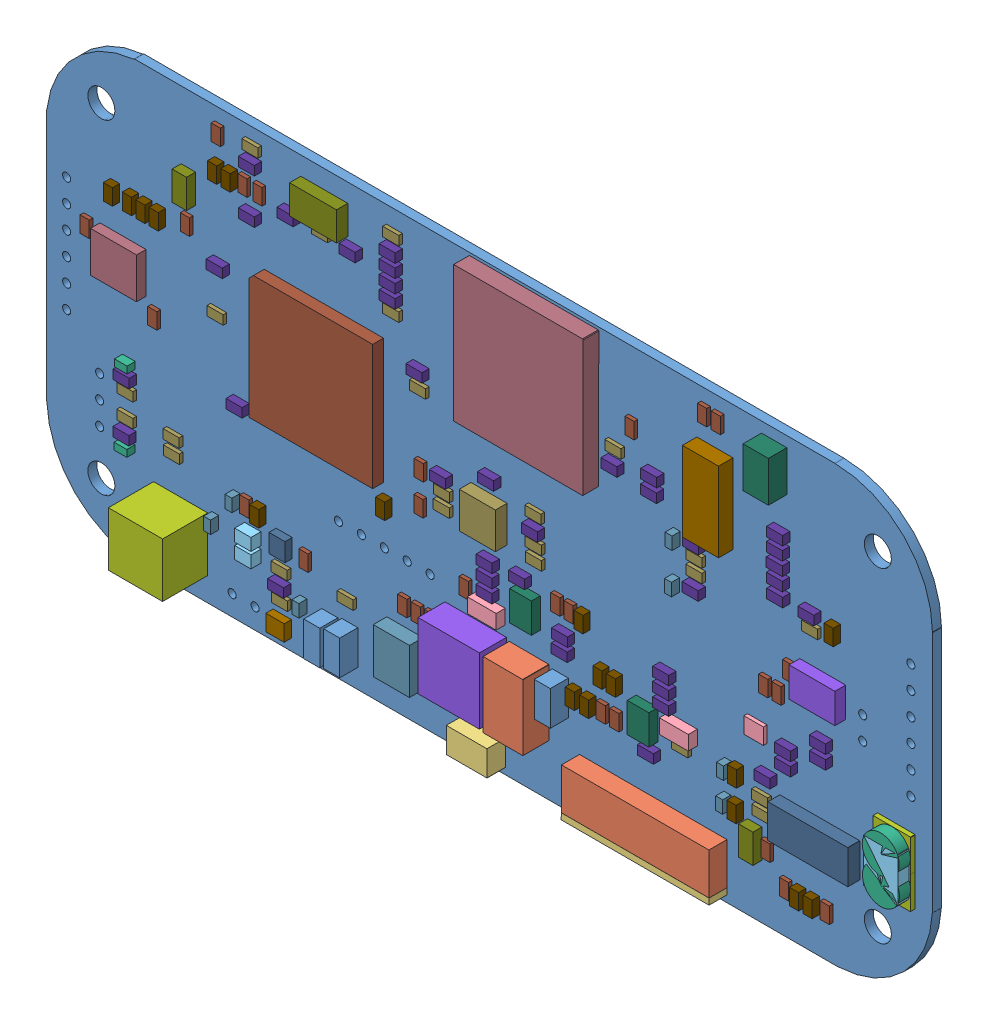
SolidWorks assembly Smart-Car, configuration 默认. Lengths in mm.
Overall size (98.16 48.13 6).
470 component instances, 34 part files, 0 mates.
Components (placement in the parent):
- Smart-Car.step-1: Smart-Car.step [默认] at origin size (98.16 48.13 6)
  - Board.step-1: Board.step [默认] at origin size (98.16 48.13 1)
    - Open CASCADE STEP translator 6.8 1.1.1.step-1: Open CASCADE STEP translator 6.8 1.1.1.step [默认] at (0 0 -1) size (98.16 48.13 1)
  - P6.step-1: P6.step [默认] at origin size (16.38 5.29 2)
    - 5971148480.step-1: 5971148480.step [默认] at (61.1337 -2.3055 0) size (16.35 4.6 2)
      - Extruded.step-1: Extruded.step [默认] at origin size (16.35 4.6 2)
    - 5971148320.step-1: 5971148320.step [默认] at (61.1176 -4.9492 0) size (16.37 0.68 2)
      - Extruded-0.step-1: Extruded-0.step [默认] at origin size (16.37 0.68 2)
  - R49.step-1: R49.step [默认] at origin size (2.16 1.78 0.4)
    - 5971148160.step-1: 5971148160.step [默认] at (72.644 12.3266 0) size (2.16 1.78 0.4)
      - Extruded-1.step-1: Extruded-1.step [默认] at origin size (2.16 1.78 0.4)
  - Y2.step-1: Y2.step [默认] at origin size (4.18 7.17 1.73)
    - 5971145200.step-1: 5971145200.step [默认] at (88.0642 7.3026 0) size (3.8 4.84 1.73)
      - Extruded-2.step-1: Extruded-2.step [默认] at origin size (3.8 4.84 1.73)
    - 5971144960.step-1: 5971144960.step [默认] at (88.0494 8.829 0) x (0 1 0) z (0 0 1) size (4.1 4.1 1.73)
      - Cylinder.step-1: Cylinder.step [默认] at origin size (4.1 4.1 1.73)
    - 5971144960.step-2: 5971144960.step [默认] at (88.0723 5.8648 0) x (0 1 0) z (0 0 1) size (4.1 4.1 1.73)
      - Cylinder.step-1: Cylinder.step [默认] at origin size (4.1 4.1 1.73)
    - 5971144720.step-1: 5971144720.step [默认] at (88.049 7.3178 0) size (4.18 7.17 0.5)
      - Extruded-3.step-1: Extruded-3.step [默认] at origin size (4.18 7.17 0.5)
  - U9.step-1: U9.step [默认] at origin size (5.08 3.3 1.2)
    - 5971146320.step-1: 5971146320.step [默认] at (79.9008 19.7434 0) size (5.08 3.3 1.2)
      - Extruded-4.step-1: Extruded-4.step [默认] at origin size (5.08 3.3 1.2)
  - U8.step-1: U8.step [默认] at origin size (4 8.8 1.6)
    - 5994722544.step-1: 5994722544.step [默认] at (68.1071 32.6974 0.15) size (4 8.8 1.6)
      - Extruded-5.step-1: Extruded-5.step [默认] at origin size (4 8.8 1.6)
  - U7.step-1: U7.step [默认] at origin size (8.89 3.76 1.32)
    - 5971144560.step-1: 5971144560.step [默认] at (79.5515 5.3594 0) size (8.89 3.76 1.32)
      - Extruded-6.step-1: Extruded-6.step [默认] at origin size (8.89 3.76 1.32)
  - R48.step-1: R48.step [默认] at origin size (1.02 1.78 0.4)
    - 5971146720.step-1: 5971146720.step [默认] at (76.3524 19.8603 0) size (1.02 1.78 0.4)
      - Extruded-7.step-1: Extruded-7.step [默认] at origin size (1.02 1.78 0.4)
  - R47.step-1: R47.step [默认] at origin size (1.78 1.02 0.4)
    - 5971147840.step-1: 5971147840.step [默认] at (78.8391 25.0774 0) size (1.78 1.02 0.4)
      - Extruded-8.step-1: Extruded-8.step [默认] at origin size (1.78 1.02 0.4)
  - R46.step-1: R46.step [默认] at origin size (1.78 1.02 0.4)
    - 5971147840.step-1: 5971147840.step [默认] at (57.0509 31.5011 0) size (1.78 1.02 0.4)
      - Extruded-8.step-1: Extruded-8.step [默认] at origin size (1.78 1.02 0.4)
  - R45.step-1: R45.step [默认] at origin size (1.02 1.78 0.4)
    - 5971146720.step-1: 5971146720.step [默认] at (68.4454 39.7383 0) size (1.02 1.78 0.4)
      - Extruded-7.step-1: Extruded-7.step [默认] at origin size (1.02 1.78 0.4)
  - R44.step-1: R44.step [默认] at origin size (1.02 1.78 0.4)
    - 5971146720.step-1: 5971146720.step [默认] at (66.9366 39.7383 0) size (1.02 1.78 0.4)
      - Extruded-7.step-1: Extruded-7.step [默认] at origin size (1.02 1.78 0.4)
  - R43.step-1: R43.step [默认] at origin size (1.02 1.78 0.4)
    - 5971146720.step-1: 5971146720.step [默认] at (58.8975 34.4653 0) size (1.02 1.78 0.4)
      - Extruded-7.step-1: Extruded-7.step [默认] at origin size (1.02 1.78 0.4)
  - R42.step-1: R42.step [默认] at origin size (1.78 1.02 0.4)
    - 5971147840.step-1: 5971147840.step [默认] at (66.0146 24.036 0) size (1.78 1.02 0.4)
      - Extruded-8.step-1: Extruded-8.step [默认] at origin size (1.78 1.02 0.4)
  - R41.step-1: R41.step [默认] at origin size (1.78 1.02 0.4)
    - 5971147840.step-1: 5971147840.step [默认] at (66.0146 25.5143 0) size (1.78 1.02 0.4)
      - Extruded-8.step-1: Extruded-8.step [默认] at origin size (1.78 1.02 0.4)
  - R40.step-1: R40.step [默认] at origin size (1.02 1.78 0.4)
    - 5971146720.step-1: 5971146720.step [默认] at (73.9572 1.463 0) size (1.02 1.78 0.4)
      - Extruded-7.step-1: Extruded-7.step [默认] at origin size (1.02 1.78 0.4)
  - R39.step-1: R39.step [默认] at origin size (1.02 1.78 0.4)
    - 5971146720.step-1: 5971146720.step [默认] at (75.9993 -1.209 0) size (1.02 1.78 0.4)
      - Extruded-7.step-1: Extruded-7.step [默认] at origin size (1.02 1.78 0.4)
  - R38.step-1: R38.step [默认] at origin size (1.78 1.02 0.4)
    - 5971147840.step-1: 5971147840.step [默认] at (73.3044 6.1341 0) size (1.78 1.02 0.4)
      - Extruded-8.step-1: Extruded-8.step [默认] at origin size (1.78 1.02 0.4)
  - R37.step-1: R37.step [默认] at origin size (1.02 1.78 0.4)
    - 5971146720.step-1: 5971146720.step [默认] at (80.5129 -1.2116 0) size (1.02 1.78 0.4)
      - Extruded-7.step-1: Extruded-7.step [默认] at origin size (1.02 1.78 0.4)
  - R36.step-1: R36.step [默认] at origin size (1.78 1.02 0.4)
    - 5971147840.step-1: 5971147840.step [默认] at (73.3273 4.6685 0) size (1.78 1.02 0.4)
      - Extruded-8.step-1: Extruded-8.step [默认] at origin size (1.78 1.02 0.4)
  - P10.step-1: P10.step [默认] at origin size (14.38 15.03 1.73)
    - 5971145360.step-1: 5971145360.step [默认] at (47.9066 34.2417 0) size (14.38 15.03 1.73)
      - Extruded-9.step-1: Extruded-9.step [默认] at origin size (14.38 15.03 1.73)
  - ESD9.step-1: ESD9.step [默认] at origin size (0.76 1.4 0.9)
    - 5971147360.step-1: 5971147360.step [默认] at (63.6523 21.7882 0) size (0.76 1.4 0.9)
      - Extruded-10.step-1: Extruded-10.step [默认] at origin size (0.76 1.4 0.9)
  - ESD8.step-1: ESD8.step [默认] at origin size (0.76 1.4 0.9)
    - 5971147360.step-1: 5971147360.step [默认] at (63.7236 26.2686 0) size (0.76 1.4 0.9)
      - Extruded-10.step-1: Extruded-10.step [默认] at origin size (0.76 1.4 0.9)
  - ESD7.step-1: ESD7.step [默认] at origin size (0.76 1.4 0.9)
    - 5971147360.step-1: 5971147360.step [默认] at (69.4107 7.0523 0) size (0.76 1.4 0.9)
      - Extruded-10.step-1: Extruded-10.step [默认] at origin size (0.76 1.4 0.9)
  - ESD6.step-1: ESD6.step [默认] at origin size (0.76 1.4 0.9)
    - 5971147360.step-1: 5971147360.step [默认] at (69.3267 3.7706 0) size (0.76 1.4 0.9)
      - Extruded-10.step-1: Extruded-10.step [默认] at origin size (0.76 1.4 0.9)
  - D8.step-1: D8.step [默认] at origin size (2.81 4.5 2.05)
    - 5971148000.step-1: 5971148000.step [默认] at (74.5249 38.655 0) size (2.81 4.5 2.05)
      - Extruded-11.step-1: Extruded-11.step [默认] at origin size (2.81 4.5 2.05)
  - D7.step-1: D7.step [默认] at origin size (1.6 3.2 1)
    - 5994722384.step-1: 5994722384.step [默认] at (72.3621 1.5426 0) size (1.6 3.2 1)
      - Extruded-12.step-1: Extruded-12.step [默认] at origin size (1.6 3.2 1)
  - C66.step-1: C66.step [默认] at origin size (1.78 1.02 0.8)
    - 5971147680.step-1: 5971147680.step [默认] at (75.3313 28.1178 0) size (1.78 1.02 0.8)
      - Extruded-13.step-1: Extruded-13.step [默认] at origin size (1.78 1.02 0.8)
  - C65.step-1: C65.step [默认] at origin size (1.78 1.02 0.8)
    - 5971147680.step-1: 5971147680.step [默认] at (80.1091 14.9098 0) size (1.78 1.02 0.8)
      - Extruded-13.step-1: Extruded-13.step [默认] at origin size (1.78 1.02 0.8)
  - C64.step-1: C64.step [默认] at origin size (1.78 1.02 0.8)
    - 5971147680.step-1: 5971147680.step [默认] at (80.1091 13.401 0) size (1.78 1.02 0.8)
      - Extruded-13.step-1: Extruded-13.step [默认] at origin size (1.78 1.02 0.8)
  - C63.step-1: C63.step [默认] at origin size (1.78 1.02 0.8)
    - 5971147680.step-1: 5971147680.step [默认] at (75.3669 26.5989 0) size (1.78 1.02 0.8)
      - Extruded-13.step-1: Extruded-13.step [默认] at origin size (1.78 1.02 0.8)
  - C62.step-1: C62.step [默认] at origin size (1.78 1.02 0.8)
    - 5971147680.step-1: 5971147680.step [默认] at (78.8238 26.609 0) size (1.78 1.02 0.8)
      - Extruded-13.step-1: Extruded-13.step [默认] at origin size (1.78 1.02 0.8)
  - C61.step-1: C61.step [默认] at origin size (1.02 1.78 0.8)
    - 5971146160.step-1: 5971146160.step [默认] at (81.346 26.0528 0) size (1.02 1.78 0.8)
      - Extruded-14.step-1: Extruded-14.step [默认] at origin size (1.02 1.78 0.8)
  - C60.step-1: C60.step [默认] at origin size (1.78 1.02 0.8)
    - 5971147680.step-1: 5971147680.step [默认] at (57.0154 29.9491 0) size (1.78 1.02 0.8)
      - Extruded-13.step-1: Extruded-13.step [默认] at origin size (1.78 1.02 0.8)
  - C59.step-1: C59.step [默认] at origin size (1.78 1.02 0.8)
    - 5971147680.step-1: 5971147680.step [默认] at (66.0146 22.5577 0) size (1.78 1.02 0.8)
      - Extruded-13.step-1: Extruded-13.step [默认] at origin size (1.78 1.02 0.8)
  - C58.step-1: C58.step [默认] at origin size (1.78 1.02 0.8)
    - 5971147680.step-1: 5971147680.step [默认] at (75.3262 29.591 0) size (1.78 1.02 0.8)
      - Extruded-13.step-1: Extruded-13.step [默认] at origin size (1.78 1.02 0.8)
  - C57.step-1: C57.step [默认] at origin size (1.78 1.02 0.8)
    - 5971147680.step-1: 5971147680.step [默认] at (75.3339 31.0693 0) size (1.78 1.02 0.8)
      - Extruded-13.step-1: Extruded-13.step [默认] at origin size (1.78 1.02 0.8)
  - C56.step-1: C56.step [默认] at origin size (1.78 1.02 0.8)
    - 5971147680.step-1: 5971147680.step [默认] at (75.3567 32.5298 0) size (1.78 1.02 0.8)
      - Extruded-13.step-1: Extruded-13.step [默认] at origin size (1.78 1.02 0.8)
  - C55.step-1: C55.step [默认] at origin size (1.78 1.02 0.8)
    - 5971147680.step-1: 5971147680.step [默认] at (61.4197 31.1277 0) size (1.78 1.02 0.8)
      - Extruded-13.step-1: Extruded-13.step [默认] at origin size (1.78 1.02 0.8)
  - C54.step-1: C54.step [默认] at origin size (1.78 1.02 0.8)
    - 5971147680.step-1: 5971147680.step [默认] at (66.0324 27.0104 0) size (1.78 1.02 0.8)
      - Extruded-13.step-1: Extruded-13.step [默认] at origin size (1.78 1.02 0.8)
  - C53.step-1: C53.step [默认] at origin size (1.78 1.02 0.8)
    - 5971147680.step-1: 5971147680.step [默认] at (61.3943 29.6189 0) size (1.78 1.02 0.8)
      - Extruded-13.step-1: Extruded-13.step [默认] at origin size (1.78 1.02 0.8)
  - C52.step-1: C52.step [默认] at origin size (1.02 1.78 0.8)
    - 5971146160.step-1: 5971146160.step [默认] at (70.6298 7.1247 0) size (1.02 1.78 0.8)
      - Extruded-14.step-1: Extruded-14.step [默认] at origin size (1.02 1.78 0.8)
  - C51.step-1: C51.step [默认] at origin size (1.78 1.02 0.8)
    - 5971147680.step-1: 5971147680.step [默认] at (73.9445 8.5141 0) size (1.78 1.02 0.8)
      - Extruded-13.step-1: Extruded-13.step [默认] at origin size (1.78 1.02 0.8)
  - C50.step-1: C50.step [默认] at origin size (1.78 1.02 0.8)
    - 5971147680.step-1: 5971147680.step [默认] at (76.2203 10.8026 0) size (1.78 1.02 0.8)
      - Extruded-13.step-1: Extruded-13.step [默认] at origin size (1.78 1.02 0.8)
  - C49.step-1: C49.step [默认] at origin size (1.02 1.78 0.8)
    - 5971146160.step-1: 5971146160.step [默认] at (77.5208 -1.209 0) size (1.02 1.78 0.8)
      - Extruded-14.step-1: Extruded-14.step [默认] at origin size (1.02 1.78 0.8)
  - C48.step-1: C48.step [默认] at origin size (1.78 1.02 0.8)
    - 5971147680.step-1: 5971147680.step [默认] at (76.2305 12.2758 0) size (1.78 1.02 0.8)
      - Extruded-13.step-1: Extruded-13.step [默认] at origin size (1.78 1.02 0.8)
  - C47.step-1: C47.step [默认] at origin size (1.02 1.78 0.8)
    - 5971146160.step-1: 5971146160.step [默认] at (79.0143 -1.1989 0) size (1.02 1.78 0.8)
      - Extruded-14.step-1: Extruded-14.step [默认] at origin size (1.02 1.78 0.8)
  - C46.step-1: C46.step [默认] at origin size (1.02 1.78 0.8)
    - 5971146160.step-1: 5971146160.step [默认] at (70.5891 3.6957 0) size (1.02 1.78 0.8)
      - Extruded-14.step-1: Extruded-14.step [默认] at origin size (1.02 1.78 0.8)
  - C1.step-1: C1.step [默认] at origin size (1.78 1.02 0.8)
    - 5971147680.step-1: 5971147680.step [默认] at (16.8524 38.7674 0) size (1.78 1.02 0.8)
      - Extruded-13.step-1: Extruded-13.step [默认] at origin size (1.78 1.02 0.8)
  - C2.step-1: C2.step [默认] at origin size (1.02 1.78 0.8)
    - 5971146160.step-1: 5971146160.step [默认] at (31.6733 13.3115 0) size (1.02 1.78 0.8)
      - Extruded-14.step-1: Extruded-14.step [默认] at origin size (1.02 1.78 0.8)
  - C3.step-1: C3.step [默认] at origin size (1.78 1.02 0.8)
    - 5971147680.step-1: 5971147680.step [默认] at (15.496 14.866 0) size (1.78 1.02 0.8)
      - Extruded-13.step-1: Extruded-13.step [默认] at origin size (1.78 1.02 0.8)
  - C4.step-1: C4.step [默认] at origin size (1.78 1.02 0.8)
    - 5971147680.step-1: 5971147680.step [默认] at (13.3015 27.1469 0) size (1.78 1.02 0.8)
      - Extruded-13.step-1: Extruded-13.step [默认] at origin size (1.78 1.02 0.8)
  - C5.step-1: C5.step [默认] at origin size (1.78 1.02 0.8)
    - 5971147680.step-1: 5971147680.step [默认] at (32.4505 35.247 0) size (1.78 1.02 0.8)
      - Extruded-13.step-1: Extruded-13.step [默认] at origin size (1.78 1.02 0.8)
  - C6.step-1: C6.step [默认] at origin size (1.78 1.02 0.8)
    - 5971147680.step-1: 5971147680.step [默认] at (35.4172 28.1731 0) size (1.78 1.02 0.8)
      - Extruded-13.step-1: Extruded-13.step [默认] at origin size (1.78 1.02 0.8)
  - C7.step-1: C7.step [默认] at origin size (1.78 1.02 0.8)
    - 5971147680.step-1: 5971147680.step [默认] at (28.0131 36.0191 0) size (1.78 1.02 0.8)
      - Extruded-13.step-1: Extruded-13.step [默认] at origin size (1.78 1.02 0.8)
  - C8.step-1: C8.step [默认] at origin size (1.78 1.02 0.8)
    - 5971147680.step-1: 5971147680.step [默认] at (21.1399 36.0394 0) size (1.78 1.02 0.8)
      - Extruded-13.step-1: Extruded-13.step [默认] at origin size (1.78 1.02 0.8)
  - C9.step-1: C9.step [默认] at origin size (1.78 1.02 0.8)
    - 5971147680.step-1: 5971147680.step [默认] at (32.4505 33.7865 0) size (1.78 1.02 0.8)
      - Extruded-13.step-1: Extruded-13.step [默认] at origin size (1.78 1.02 0.8)
  - C10.step-1: C10.step [默认] at origin size (1.78 1.02 0.8)
    - 5971147680.step-1: 5971147680.step [默认] at (32.4505 36.7303 0) size (1.78 1.02 0.8)
      - Extruded-13.step-1: Extruded-13.step [默认] at origin size (1.78 1.02 0.8)
  - C11.step-1: C11.step [默认] at origin size (1.78 1.02 0.8)
    - 5971147680.step-1: 5971147680.step [默认] at (32.4505 38.1857 0) size (1.78 1.02 0.8)
      - Extruded-13.step-1: Extruded-13.step [默认] at origin size (1.78 1.02 0.8)
  - C12.step-1: C12.step [默认] at origin size (1.02 1.78 0.8)
    - 5971146160.step-1: 5971146160.step [默认] at (14.5537 36.2604 0) size (1.02 1.78 0.8)
      - Extruded-14.step-1: Extruded-14.step [默认] at origin size (1.02 1.78 0.8)
  - C13.step-1: C13.step [默认] at origin size (1.02 1.78 0.8)
    - 5971146160.step-1: 5971146160.step [默认] at (13.0627 36.2604 0) size (1.02 1.78 0.8)
      - Extruded-14.step-1: Extruded-14.step [默认] at origin size (1.02 1.78 0.8)
  - C14.step-1: C14.step [默认] at origin size (1.78 1.02 0.8)
    - 5971147680.step-1: 5971147680.step [默认] at (16.8549 33.8347 0) size (1.78 1.02 0.8)
      - Extruded-13.step-1: Extruded-13.step [默认] at origin size (1.78 1.02 0.8)
  - C15.step-1: C15.step [默认] at origin size (1.78 1.02 0.8)
    - 5971147680.step-1: 5971147680.step [默认] at (43.3446 21.7687 0) size (1.78 1.02 0.8)
      - Extruded-13.step-1: Extruded-13.step [默认] at origin size (1.78 1.02 0.8)
  - C16.step-1: C16.step [默认] at origin size (1.78 1.02 0.8)
    - 5971147680.step-1: 5971147680.step [默认] at (38.0233 19.3075 0) size (1.78 1.02 0.8)
      - Extruded-13.step-1: Extruded-13.step [默认] at origin size (1.78 1.02 0.8)
  - C17.step-1: C17.step [默认] at origin size (1.78 1.02 0.8)
    - 5971147680.step-1: 5971147680.step [默认] at (48.2138 19.31 0) size (1.78 1.02 0.8)
      - Extruded-13.step-1: Extruded-13.step [默认] at origin size (1.78 1.02 0.8)
  - C18.step-1: C18.step [默认] at origin size (1.78 1.02 0.8)
    - 5971147680.step-1: 5971147680.step [默认] at (2.9947 11.4325 0) size (1.78 1.02 0.8)
      - Extruded-13.step-1: Extruded-13.step [默认] at origin size (1.78 1.02 0.8)
  - C19.step-1: C19.step [默认] at origin size (1.02 1.78 0.8)
    - 5971146160.step-1: 5971146160.step [默认] at (1.5189 28.3945 0) size (1.02 1.78 0.8)
      - Extruded-14.step-1: Extruded-14.step [默认] at origin size (1.02 1.78 0.8)
  - C20.step-1: C20.step [默认] at origin size (1.78 1.02 0.8)
    - 5971147680.step-1: 5971147680.step [默认] at (2.9616 5.9157 0) size (1.78 1.02 0.8)
      - Extruded-13.step-1: Extruded-13.step [默认] at origin size (1.78 1.02 0.8)
  - C21.step-1: C21.step [默认] at origin size (1.02 1.78 0.8)
    - 5971146160.step-1: 5971146160.step [默认] at (3.6271 28.5369 0) size (1.02 1.78 0.8)
      - Extruded-14.step-1: Extruded-14.step [默认] at origin size (1.02 1.78 0.8)
  - C22.step-1: C22.step [默认] at origin size (1.02 1.78 0.8)
    - 5971146160.step-1: 5971146160.step [默认] at (5.1156 28.5316 0) size (1.02 1.78 0.8)
      - Extruded-14.step-1: Extruded-14.step [默认] at origin size (1.02 1.78 0.8)
  - C23.step-1: C23.step [默认] at origin size (1.02 1.78 0.8)
    - 5971146160.step-1: 5971146160.step [默认] at (6.5938 28.552 0) size (1.02 1.78 0.8)
      - Extruded-14.step-1: Extruded-14.step [默认] at origin size (1.02 1.78 0.8)
  - C24.step-1: C24.step [默认] at origin size (1.78 1.02 0.8)
    - 5971147680.step-1: 5971147680.step [默认] at (39.7606 -1.5983 0) size (1.78 1.02 0.8)
      - Extruded-13.step-1: Extruded-13.step [默认] at origin size (1.78 1.02 0.8)
  - C25.step-1: C25.step [默认] at origin size (1.02 1.78 0.8)
    - 5971146160.step-1: 5971146160.step [默认] at (52.6842 5.5975 0) size (1.02 1.78 0.8)
      - Extruded-14.step-1: Extruded-14.step [默认] at origin size (1.02 1.78 0.8)
  - C26.step-1: C26.step [默认] at origin size (1.78 3.81 2)
    - 5994723424.step-1: 5994723424.step [默认] at (50.8325 4.7912 0) size (1.78 3.81 2)
      - Extruded-15.step-1: Extruded-15.step [默认] at origin size (1.78 3.81 2)
  - C27.step-1: C27.step [默认] at origin size (1.78 3.81 2)
    - 5994723424.step-1: 5994723424.step [默认] at (25.3004 -2.185 0) size (1.78 3.81 2)
      - Extruded-15.step-1: Extruded-15.step [默认] at origin size (1.78 3.81 2)
  - C28.step-1: C28.step [默认] at origin size (1.78 3.81 2)
    - 5994723424.step-1: 5994723424.step [默认] at (27.5102 -2.0287 0) size (1.78 3.81 2)
      - Extruded-15.step-1: Extruded-15.step [默认] at origin size (1.78 3.81 2)
  - C29.step-1: C29.step [默认] at origin size (4.4 7.32 2.9)
    - 5994723824.step-1: 5994723824.step [默认] at (47.3781 3.2947 0) size (4.4 7.32 2.9)
      - Extruded-16.step-1: Extruded-16.step [默认] at origin size (4.4 7.32 2.9)
  - C30.step-1: C30.step [默认] at origin size (1.78 1.02 0.8)
    - 5971147680.step-1: 5971147680.step [默认] at (51.5361 10.8858 0) size (1.78 1.02 0.8)
      - Extruded-13.step-1: Extruded-13.step [默认] at origin size (1.78 1.02 0.8)
  - C31.step-1: C31.step [默认] at origin size (1.78 1.02 0.8)
    - 5971147680.step-1: 5971147680.step [默认] at (51.5056 9.4228 0) size (1.78 1.02 0.8)
      - Extruded-13.step-1: Extruded-13.step [默认] at origin size (1.78 1.02 0.8)
  - C32.step-1: C32.step [默认] at origin size (1.78 1.02 0.8)
    - 5971147680.step-1: 5971147680.step [默认] at (43.1541 10.8655 0) size (1.78 1.02 0.8)
      - Extruded-13.step-1: Extruded-13.step [默认] at origin size (1.78 1.02 0.8)
  - C33.step-1: C33.step [默认] at origin size (1.78 1.02 0.8)
    - 5971147680.step-1: 5971147680.step [默认] at (43.1719 12.3235 0) size (1.78 1.02 0.8)
      - Extruded-13.step-1: Extruded-13.step [默认] at origin size (1.78 1.02 0.8)
  - C34.step-1: C34.step [默认] at origin size (1.78 1.02 0.8)
    - 5971147680.step-1: 5971147680.step [默认] at (43.1896 13.7916 0) size (1.78 1.02 0.8)
      - Extruded-13.step-1: Extruded-13.step [默认] at origin size (1.78 1.02 0.8)
  - C35.step-1: C35.step [默认] at origin size (1.02 1.78 0.8)
    - 5971146160.step-1: 5971146160.step [默认] at (53.6341 13.4334 0) size (1.02 1.78 0.8)
      - Extruded-14.step-1: Extruded-14.step [默认] at origin size (1.02 1.78 0.8)
  - C36.step-1: C36.step [默认] at origin size (1.78 1.02 0.8)
    - 5971147680.step-1: 5971147680.step [默认] at (46.7766 14.0437 0) size (1.78 1.02 0.8)
      - Extruded-13.step-1: Extruded-13.step [默认] at origin size (1.78 1.02 0.8)
  - C37.step-1: C37.step [默认] at origin size (1.78 1.02 0.8)
    - 5971147680.step-1: 5971147680.step [默认] at (20.101 -0.1124 0) size (1.78 1.02 0.8)
      - Extruded-13.step-1: Extruded-13.step [默认] at origin size (1.78 1.02 0.8)
  - C38.step-1: C38.step [默认] at origin size (1.02 1.78 0.8)
    - 5971146160.step-1: 5971146160.step [默认] at (17.7236 5.6229 0) size (1.02 1.78 0.8)
      - Extruded-14.step-1: Extruded-14.step [默认] at origin size (1.02 1.78 0.8)
  - C39.step-1: C39.step [默认] at origin size (1.02 1.78 0.8)
    - 5971146160.step-1: 5971146160.step [默认] at (55.7347 9.1561 0) size (1.02 1.78 0.8)
      - Extruded-14.step-1: Extruded-14.step [默认] at origin size (1.02 1.78 0.8)
  - C40.step-1: C40.step [默认] at origin size (1.02 1.78 0.8)
    - 5971146160.step-1: 5971146160.step [默认] at (57.2231 9.1434 0) size (1.02 1.78 0.8)
      - Extruded-14.step-1: Extruded-14.step [默认] at origin size (1.02 1.78 0.8)
  - C41.step-1: C41.step [默认] at origin size (1.78 1.02 0.8)
    - 5971147680.step-1: 5971147680.step [默认] at (62.74 9.8774 0) size (1.78 1.02 0.8)
      - Extruded-13.step-1: Extruded-13.step [默认] at origin size (1.78 1.02 0.8)
  - C42.step-1: C42.step [默认] at origin size (1.78 1.02 0.8)
    - 5971147680.step-1: 5971147680.step [默认] at (62.7349 11.3506 0) size (1.78 1.02 0.8)
      - Extruded-13.step-1: Extruded-13.step [默认] at origin size (1.78 1.02 0.8)
  - C43.step-1: C43.step [默认] at origin size (1.78 1.02 0.8)
    - 5971147680.step-1: 5971147680.step [默认] at (62.7476 12.8111 0) size (1.78 1.02 0.8)
      - Extruded-13.step-1: Extruded-13.step [默认] at origin size (1.78 1.02 0.8)
  - C44.step-1: C44.step [默认] at origin size (1.02 1.78 0.8)
    - 5971146160.step-1: 5971146160.step [默认] at (54.2539 5.6179 0) size (1.02 1.78 0.8)
      - Extruded-14.step-1: Extruded-14.step [默认] at origin size (1.02 1.78 0.8)
  - C45.step-1: C45.step [默认] at origin size (1.78 1.02 0.8)
    - 5971147680.step-1: 5971147680.step [默认] at (61.056 4.4469 0) size (1.78 1.02 0.8)
      - Extruded-13.step-1: Extruded-13.step [默认] at origin size (1.78 1.02 0.8)
  - D1.step-1: D1.step [默认] at origin size (1.6 3.2 1)
    - 5994722384.step-1: 5994722384.step [默认] at (9.6317 32.9912 0) size (1.6 3.2 1)
      - Extruded-12.step-1: Extruded-12.step [默认] at origin size (1.6 3.2 1)
  - D2.step-1: D2.step [默认] at origin size (4.5 2.81 2.05)
    - 5994723664.step-1: 5994723664.step [默认] at (42.5037 -3.9434 0) size (4.5 2.81 2.05)
      - Extruded-17.step-1: Extruded-17.step [默认] at origin size (4.5 2.81 2.05)
  - D3.step-1: D3.step [默认] at origin size (3.2 1.6 1)
    - 5994721984.step-1: 5994721984.step [默认] at (43.1253 9.1027 0) size (3.2 1.6 1)
      - Extruded-18.step-1: Extruded-18.step [默认] at origin size (3.2 1.6 1)
  - D4.step-1: D4.step [默认] at origin size (1.8 1.35 1.1)
    - 5994721664.step-1: 5994721664.step [默认] at (16.7609 1.3659 0) size (1.8 1.35 1.1)
      - Extruded-19.step-1: Extruded-19.step [默认] at origin size (1.8 1.35 1.1)
  - D5.step-1: D5.step [默认] at origin size (1.8 1.35 1.1)
    - 5994721664.step-1: 5994721664.step [默认] at (16.766 3.0347 0) size (1.8 1.35 1.1)
      - Extruded-19.step-1: Extruded-19.step [默认] at origin size (1.8 1.35 1.1)
  - D6.step-1: D6.step [默认] at origin size (3.2 1.6 1)
    - 5994721984.step-1: 5994721984.step [默认] at (64.4071 8.1375 0) size (3.2 1.6 1)
      - Extruded-18.step-1: Extruded-18.step [默认] at origin size (3.2 1.6 1)
  - ESD1.step-1: ESD1.step [默认] at origin size (1.4 0.76 0.9)
    - 5971140800.step-1: 5971140800.step [默认] at (3.0467 12.7052 0) size (1.4 0.76 0.9)
      - Extruded-20.step-1: Extruded-20.step [默认] at origin size (1.4 0.76 0.9)
  - ESD2.step-1: ESD2.step [默认] at origin size (1.4 0.76 0.9)
    - 5971140800.step-1: 5971140800.step [默认] at (3.0162 4.6965 0) size (1.4 0.76 0.9)
      - Extruded-20.step-1: Extruded-20.step [默认] at origin size (1.4 0.76 0.9)
  - ESD3.step-1: ESD3.step [默认] at origin size (0.76 1.4 0.9)
    - 5971147360.step-1: 5971147360.step [默认] at (22.3844 -0.8833 0) size (0.76 1.4 0.9)
      - Extruded-10.step-1: Extruded-10.step [默认] at origin size (0.76 1.4 0.9)
  - ESD4.step-1: ESD4.step [默认] at origin size (0.76 1.4 0.9)
    - 5971147360.step-1: 5971147360.step [默认] at (14.9779 5.5252 0) size (0.76 1.4 0.9)
      - Extruded-10.step-1: Extruded-10.step [默认] at origin size (0.76 1.4 0.9)
  - ESD5.step-1: ESD5.step [默认] at origin size (0.76 1.4 0.9)
    - 5971147360.step-1: 5971147360.step [默认] at (12.6105 2.2423 0) size (0.76 1.4 0.9)
      - Extruded-10.step-1: Extruded-10.step [默认] at origin size (0.76 1.4 0.9)
  - K1.step-1: K1.step [默认] at origin size (6 6 5)
    - 5994726224.step-1: 5994726224.step [默认] at (8.7795 -0.4263 0) size (6 6 5)
      - Extruded-21.step-1: Extruded-21.step [默认] at origin size (6 6 5)
  - L1.step-1: L1.step [默认] at origin size (1.78 1.02 0.4)
    - 5971147840.step-1: 5971147840.step [默认] at (32.4505 39.6564 0) size (1.78 1.02 0.4)
      - Extruded-8.step-1: Extruded-8.step [默认] at origin size (1.78 1.02 0.4)
  - L2.step-1: L2.step [默认] at origin size (1.02 1.78 0.4)
    - 5971146720.step-1: 5971146720.step [默认] at (13.0627 39.6843 0) size (1.02 1.78 0.4)
      - Extruded-7.step-1: Extruded-7.step [默认] at origin size (1.02 1.78 0.4)
  - L3.step-1: L3.step [默认] at origin size (6.81 7.32 3)
    - 5994722944.step-1: 5994722944.step [默认] at (41.4675 3.5312 0) size (6.81 7.32 3)
      - Extruded-22.step-1: Extruded-22.step [默认] at origin size (6.81 7.32 3)
  - Q1.step-1: Q1.step [默认] at origin size (2.03 1.78 0.8)
    - 5994724624.step-1: 5994724624.step [默认] at (20.0299 -3.9148 0) size (2.03 1.78 0.8)
      - Extruded-23.step-1: Extruded-23.step [默认] at origin size (2.03 1.78 0.8)
  - Q2.step-1: Q2.step [默认] at origin size (1.78 2.03 0.8)
    - 5994725744.step-1: 5994725744.step [默认] at (20.2484 3.883 0) size (1.78 2.03 0.8)
      - Extruded-24.step-1: Extruded-24.step [默认] at origin size (1.78 2.03 0.8)
  - R1.step-1: R1.step [默认] at origin size (1.78 1.02 0.4)
    - 5971147840.step-1: 5971147840.step [默认] at (16.8397 40.2584 0) size (1.78 1.02 0.4)
      - Extruded-8.step-1: Extruded-8.step [默认] at origin size (1.78 1.02 0.4)
  - R2.step-1: R2.step [默认] at origin size (1.78 1.02 0.4)
    - 5971147840.step-1: 5971147840.step [默认] at (35.4101 26.4338 0) size (1.78 1.02 0.4)
      - Extruded-8.step-1: Extruded-8.step [默认] at origin size (1.78 1.02 0.4)
  - R3.step-1: R3.step [默认] at origin size (1.78 1.02 0.4)
    - 5971147840.step-1: 5971147840.step [默认] at (12.9946 22.3291 0) size (1.78 1.02 0.4)
      - Extruded-8.step-1: Extruded-8.step [默认] at origin size (1.78 1.02 0.4)
  - R4.step-1: R4.step [默认] at origin size (1.78 1.02 0.4)
    - 5971147840.step-1: 5971147840.step [默认] at (24.5562 36.0191 0) size (1.78 1.02 0.4)
      - Extruded-8.step-1: Extruded-8.step [默认] at origin size (1.78 1.02 0.4)
  - R5.step-1: R5.step [默认] at origin size (1.78 1.02 0.4)
    - 5971147840.step-1: 5971147840.step [默认] at (32.4505 32.3183 0) size (1.78 1.02 0.4)
      - Extruded-8.step-1: Extruded-8.step [默认] at origin size (1.78 1.02 0.4)
  - R6.step-1: R6.step [默认] at origin size (1.02 1.78 0.4)
    - 5971146720.step-1: 5971146720.step [默认] at (16.0294 36.3011 0) size (1.02 1.78 0.4)
      - Extruded-7.step-1: Extruded-7.step [默认] at origin size (1.02 1.78 0.4)
  - R7.step-1: R7.step [默认] at origin size (1.02 1.78 0.4)
    - 5971146720.step-1: 5971146720.step [默认] at (17.6753 36.2833 0) size (1.02 1.78 0.4)
      - Extruded-7.step-1: Extruded-7.step [默认] at origin size (1.02 1.78 0.4)
  - R8.step-1: R8.step [默认] at origin size (1.02 1.78 0.4)
    - 5971146720.step-1: 5971146720.step [默认] at (35.5493 18.7487 0) size (1.02 1.78 0.4)
      - Extruded-7.step-1: Extruded-7.step [默认] at origin size (1.02 1.78 0.4)
  - R9.step-1: R9.step [默认] at origin size (1.78 1.02 0.4)
    - 5971147840.step-1: 5971147840.step [默认] at (38.0614 17.8216 0) size (1.78 1.02 0.4)
      - Extruded-8.step-1: Extruded-8.step [默认] at origin size (1.78 1.02 0.4)
  - R10.step-1: R10.step [默认] at origin size (1.78 1.02 0.4)
    - 5971147840.step-1: 5971147840.step [默认] at (8.1458 6.543 0) size (1.78 1.02 0.4)
      - Extruded-8.step-1: Extruded-8.step [默认] at origin size (1.78 1.02 0.4)
  - R11.step-1: R11.step [默认] at origin size (1.02 1.78 0.4)
    - 5971146720.step-1: 5971146720.step [默认] at (35.5214 15.2841 0) size (1.02 1.78 0.4)
      - Extruded-7.step-1: Extruded-7.step [默认] at origin size (1.02 1.78 0.4)
  - R12.step-1: R12.step [默认] at origin size (1.78 1.02 0.4)
    - 5971147840.step-1: 5971147840.step [默认] at (38.0436 16.323 0) size (1.78 1.02 0.4)
      - Extruded-8.step-1: Extruded-8.step [默认] at origin size (1.78 1.02 0.4)
  - R13.step-1: R13.step [默认] at origin size (1.78 1.02 0.4)
    - 5971147840.step-1: 5971147840.step [默认] at (48.1985 20.7908 0) size (1.78 1.02 0.4)
      - Extruded-8.step-1: Extruded-8.step [默认] at origin size (1.78 1.02 0.4)
  - R14.step-1: R14.step [默认] at origin size (1.78 1.02 0.4)
    - 5971147840.step-1: 5971147840.step [默认] at (48.2341 17.8368 0) size (1.78 1.02 0.4)
      - Extruded-8.step-1: Extruded-8.step [默认] at origin size (1.78 1.02 0.4)
  - R15.step-1: R15.step [默认] at origin size (1.78 1.02 0.4)
    - 5971147840.step-1: 5971147840.step [默认] at (8.1305 8.0874 0) size (1.78 1.02 0.4)
      - Extruded-8.step-1: Extruded-8.step [默认] at origin size (1.78 1.02 0.4)
  - R16.step-1: R16.step [默认] at origin size (1.78 1.02 0.4)
    - 5971147840.step-1: 5971147840.step [默认] at (48.2417 16.356 0) size (1.78 1.02 0.4)
      - Extruded-8.step-1: Extruded-8.step [默认] at origin size (1.78 1.02 0.4)
  - R17.step-1: R17.step [默认] at origin size (1.78 1.02 0.4)
    - 5971147840.step-1: 5971147840.step [默认] at (3.0048 9.9543 0) size (1.78 1.02 0.4)
      - Extruded-8.step-1: Extruded-8.step [默认] at origin size (1.78 1.02 0.4)
  - R18.step-1: R18.step [默认] at origin size (1.02 1.78 0.4)
    - 5971146720.step-1: 5971146720.step [默认] at (-1.4529 23.6093 0) size (1.02 1.78 0.4)
      - Extruded-7.step-1: Extruded-7.step [默认] at origin size (1.02 1.78 0.4)
  - R19.step-1: R19.step [默认] at origin size (1.78 1.02 0.4)
    - 5971147840.step-1: 5971147840.step [默认] at (2.9921 7.3838 0) size (1.78 1.02 0.4)
      - Extruded-8.step-1: Extruded-8.step [默认] at origin size (1.78 1.02 0.4)
  - R20.step-1: R20.step [默认] at origin size (1.02 1.78 0.4)
    - 5971146720.step-1: 5971146720.step [默认] at (9.6494 29.37 0) size (1.02 1.78 0.4)
      - Extruded-7.step-1: Extruded-7.step [默认] at origin size (1.02 1.78 0.4)
  - R21.step-1: R21.step [默认] at origin size (1.02 1.78 0.4)
    - 5971146720.step-1: 5971146720.step [默认] at (6.0427 18.5674 0) size (1.02 1.78 0.4)
      - Extruded-7.step-1: Extruded-7.step [默认] at origin size (1.02 1.78 0.4)
  - R22.step-1: R22.step [默认] at origin size (1.78 1.02 0.4)
    - 5971147840.step-1: 5971147840.step [默认] at (27.3934 2.1711 0) size (1.78 1.02 0.4)
      - Extruded-8.step-1: Extruded-8.step [默认] at origin size (1.78 1.02 0.4)
  - R23.step-1: R23.step [默认] at origin size (1.02 1.78 0.4)
    - 5971146720.step-1: 5971146720.step [默认] at (36.6847 4.8279 0) size (1.02 1.78 0.4)
      - Extruded-7.step-1: Extruded-7.step [默认] at origin size (1.02 1.78 0.4)
  - R24.step-1: R24.step [默认] at origin size (1.02 1.78 0.4)
    - 5971146720.step-1: 5971146720.step [默认] at (35.2242 4.8203 0) size (1.02 1.78 0.4)
      - Extruded-7.step-1: Extruded-7.step [默认] at origin size (1.02 1.78 0.4)
  - R25.step-1: R25.step [默认] at origin size (1.02 1.78 0.4)
    - 5971146720.step-1: 5971146720.step [默认] at (33.7281 4.8203 0) size (1.02 1.78 0.4)
      - Extruded-7.step-1: Extruded-7.step [默认] at origin size (1.02 1.78 0.4)
  - R26.step-1: R26.step [默认] at origin size (1.02 1.78 0.4)
    - 5971146720.step-1: 5971146720.step [默认] at (50.6776 13.4411 0) size (1.02 1.78 0.4)
      - Extruded-7.step-1: Extruded-7.step [默认] at origin size (1.02 1.78 0.4)
  - R27.step-1: R27.step [默认] at origin size (1.02 1.78 0.4)
    - 5971146720.step-1: 5971146720.step [默认] at (16.2275 5.6001 0) size (1.02 1.78 0.4)
      - Extruded-7.step-1: Extruded-7.step [默认] at origin size (1.02 1.78 0.4)
  - R28.step-1: R28.step [默认] at origin size (1.02 1.78 0.4)
    - 5971146720.step-1: 5971146720.step [默认] at (52.1431 13.4157 0) size (1.02 1.78 0.4)
      - Extruded-7.step-1: Extruded-7.step [默认] at origin size (1.02 1.78 0.4)
  - R29.step-1: R29.step [默认] at origin size (1.02 1.78 0.4)
    - 5971146720.step-1: 5971146720.step [默认] at (40.5353 9.9384 0) size (1.02 1.78 0.4)
      - Extruded-7.step-1: Extruded-7.step [默认] at origin size (1.02 1.78 0.4)
  - R30.step-1: R30.step [默认] at origin size (1.78 1.02 0.4)
    - 5971147840.step-1: 5971147840.step [默认] at (20.0909 1.3634 0) size (1.78 1.02 0.4)
      - Extruded-8.step-1: Extruded-8.step [默认] at origin size (1.78 1.02 0.4)
  - R31.step-1: R31.step [默认] at origin size (1.78 1.02 0.4)
    - 5971147840.step-1: 5971147840.step [默认] at (20.1061 -1.5754 0) size (1.78 1.02 0.4)
      - Extruded-8.step-1: Extruded-8.step [默认] at origin size (1.78 1.02 0.4)
  - R32.step-1: R32.step [默认] at origin size (1.02 1.78 0.4)
    - 5971146720.step-1: 5971146720.step [默认] at (22.7782 3.6976 0) size (1.02 1.78 0.4)
      - Extruded-7.step-1: Extruded-7.step [默认] at origin size (1.02 1.78 0.4)
  - R33.step-1: R33.step [默认] at origin size (1.02 1.78 0.4)
    - 5971146720.step-1: 5971146720.step [默认] at (57.2104 5.6077 0) size (1.02 1.78 0.4)
      - Extruded-7.step-1: Extruded-7.step [默认] at origin size (1.02 1.78 0.4)
  - R34.step-1: R34.step [默认] at origin size (1.02 1.78 0.4)
    - 5971146720.step-1: 5971146720.step [默认] at (55.7169 5.6077 0) size (1.02 1.78 0.4)
      - Extruded-7.step-1: Extruded-7.step [默认] at origin size (1.02 1.78 0.4)
  - R35.step-1: R35.step [默认] at origin size (1.78 1.02 0.4)
    - 5971147840.step-1: 5971147840.step [默认] at (64.4596 6.5627 0) size (1.78 1.02 0.4)
      - Extruded-8.step-1: Extruded-8.step [默认] at origin size (1.78 1.02 0.4)
  - U1.step-1: U1.step [默认] at origin size (13.72 13.84 1.2)
    - 5971141520.step-1: 5971141520.step [默认] at (24.3886 22.1507 0) size (13.72 13.84 1.2)
      - Extruded-25.step-1: Extruded-25.step [默认] at origin size (13.72 13.84 1.2)
  - U2.step-1: U2.step [默认] at origin size (4 4 1.3)
    - 5994727184.step-1: 5994727184.step [默认] at (42.9382 18.0781 0) size (4 4 1.3)
      - Extruded-26.step-1: Extruded-26.step [默认] at origin size (4 4 1.3)
  - U3.step-1: U3.step [默认] at origin size (5.1 4.5 1.05)
    - 5994722224.step-1: 5994722224.step [默认] at (2.5425 22.3264 0.15) size (5.1 4.5 1.05)
      - Extruded-27.step-1: Extruded-27.step [默认] at origin size (5.1 4.5 1.05)
  - U4.step-1: U4.step [默认] at origin size (4 5 1.5)
    - 5994721264.step-1: 5994721264.step [默认] at (33.8678 0.2839 0.25) size (4 5 1.5)
      - Extruded-28.step-1: Extruded-28.step [默认] at origin size (4 5 1.5)
  - U5.step-1: U5.step [默认] at origin size (2.4 3.3 1)
    - 5994721824.step-1: 5994721824.step [默认] at (47.4186 11.3919 0) size (2.4 3.3 1)
      - Extruded-29.step-1: Extruded-29.step [默认] at origin size (2.4 3.3 1)
  - U6.step-1: U6.step [默认] at origin size (2.4 3.3 1)
    - 5994721824.step-1: 5994721824.step [默认] at (60.4421 7.1825 0) size (2.4 3.3 1)
      - Extruded-29.step-1: Extruded-29.step [默认] at origin size (2.4 3.3 1)
  - Y1.step-1: Y1.step [默认] at origin size (5.2 3.19 1.25)
    - 5971142320.step-1: 5971142320.step [默认] at (24.6896 38.4309 0) size (5.2 3.19 1.25)
      - Extruded-30.step-1: Extruded-30.step [默认] at origin size (5.2 3.19 1.25)
  - R50.step-1: R50.step [默认] at origin size (1.02 1.78 0.4)
    - 5971146720.step-1: 5971146720.step [默认] at (73.7006 17.1323 0) size (1.02 1.78 0.4)
      - Extruded-7.step-1: Extruded-7.step [默认] at origin size (1.02 1.78 0.4)
  - R51.step-1: R51.step [默认] at origin size (1.02 1.78 0.4)
    - 5971146720.step-1: 5971146720.step [默认] at (75.1611 17.145 0) size (1.02 1.78 0.4)
      - Extruded-7.step-1: Extruded-7.step [默认] at origin size (1.02 1.78 0.4)
